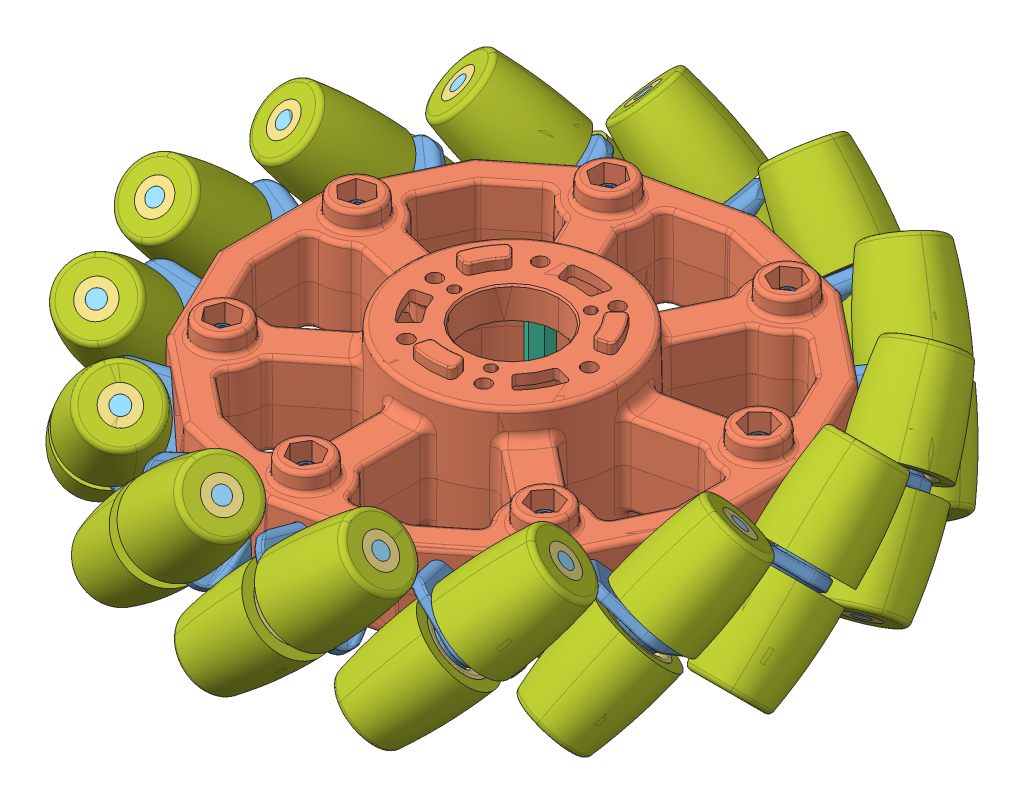
SolidWorks assembly 8_Mecanum_Wheel_Left_217-2801, configuration Default. Lengths in mm.
Overall size (213.38 67.99 218.38).
149 component instances, 10 part files, 0 mates.
Components (placement in the parent):
- 8_Mecanum_Wheel_Left_217-2801.STEP-1: 8_Mecanum_Wheel_Left_217-2801.STEP [Default] at origin size (213.38 67.99 218.38)
  - 217-2799-002 Rev1.STEP-1: 217-2799-002 Rev1.STEP [Default] at (67.5204 0 0) x (0 0 -1) z (1 0 0) size (26.84 25.28 30.1)
  - 217-2801-001 Rev1.STEP-1: 217-2801-001 Rev1.STEP [Default] at (-0.0396 6.3542 -0.0405) x (1 0 0) z (0 -1 0) size (148.4 152.01 28.7)
  - 217-2801-001 Rev1.STEP-2: 217-2801-001 Rev1.STEP [Default] at (-0.0396 -6.3458 -0.0405) x (-1 0 0) z (0 1 0) size (148.4 152.01 28.7)
  - 217-2586-003 Rev2.STEP-1: 217-2586-003 Rev2.STEP [Default] at (88.2976 -4.0062 4.0062) x (-0.854327 -0.367509 -0.367509) z (-0.519737 0.6041 0.6041) size (19.46 28.57 19.46)
  - 217-2586-003 Rev2.STEP-2: 217-2586-003 Rev2.STEP [Default] at (88.2976 4.0062 -4.0062) x (0.717269 -0.492709 -0.492709) z (0.696796 0.507186 0.507186) size (19.46 28.57 19.46)
  - 217-2586-005 Rev2.STEP-1: 217-2586-005 Rev2.STEP [Default] at (88.2976 -6.3286 6.3286) x (0 0.707107 -0.707107) z (0.473193 -0.622932 -0.622932) size (8.5 8 8)
  - 217-2586-005 Rev2.STEP-2: 217-2586-005 Rev2.STEP [Default] at (88.2976 6.3286 -6.3286) x (0 0.707107 -0.707107) z (0.707107 -0.5 -0.5) size (8.5 8 8)
  - 217-2586-007 Rev1.STEP-1: 217-2586-007 Rev1.STEP [Default] at (88.2976 0 0) x (0 0.707107 -0.707107) z (0.543569 -0.59352 -0.59352) size (61.72 5 5)
  - 217-2586-008 Rev1.STEP-1: 217-2586-008 Rev1.STEP [Default] at (-11.9459 2.5442 -20.6627) x (0.866025 0 -0.5) z (0 -1 0) size (7.33 6.35 31.75)
  - 217-2587-002 Rev2.STEP-1: 217-2587-002 Rev2.STEP [Default] at (88.2976 -0.3986 0.3986) x (-0.963241 0.189956 0.189956) z (-0.268638 -0.681114 -0.681114) size (26.1 28.56 26.1)
  - 217-2587-002 Rev2.STEP-2: 217-2587-002 Rev2.STEP [Default] at (88.2976 0.3986 -0.3986) x (0.779223 -0.443177 -0.443177) z (-0.626747 -0.550994 -0.550994) size (26.1 28.56 26.1)
  - NUT-832-NYLOCK.STEP-1: NUT-832-NYLOCK.STEP [Default] at (-49.6859 -13.6521 39.5511) x (-0.365341 0 0.930874) z (0.930874 0 0.365341) size (9.38 5.92 9.38)
  - PINL-M050-0012-S.STEP-1: PINL-M050-0012-S.STEP [Default] at (-69.318 -0.0958 -15.8528) x (0 -1 0) z (-0.272222 0 0.962235) size (12 5 5)
  - SCREW-832-1250.STEP-1: SCREW-832-1250.STEP [Default] at (-49.6859 14.914 39.5511) x (0 -1 0) z (-0.321403 0 -0.946943) size (37.06 8 10.03)
  - 217-2586-008 Rev1.STEP-2: 217-2586-008 Rev1.STEP [Default] at (-23.8521 2.5442 -0.0405) x (0 0 -1) z (0 -1 0) size (7.33 6.35 31.75)
  - 217-2586-008 Rev1.STEP-3: 217-2586-008 Rev1.STEP [Default] at (-11.9459 2.5442 20.5817) x (-0.866025 0 -0.5) z (0 -1 0) size (7.33 6.35 31.75)
  - 217-2586-008 Rev1.STEP-4: 217-2586-008 Rev1.STEP [Default] at (11.8666 2.5442 20.5817) x (-0.866025 0 0.5) z (0 -1 0) size (7.33 6.35 31.75)
  - 217-2586-008 Rev1.STEP-5: 217-2586-008 Rev1.STEP [Default] at (23.7729 2.5442 -0.0405) x (0 0 1) z (0 -1 0) size (7.33 6.35 31.75)
  - 217-2586-008 Rev1.STEP-6: 217-2586-008 Rev1.STEP [Default] at (11.8666 2.5442 -20.6627) x (0.866025 0 0.5) z (0 -1 0) size (7.33 6.35 31.75)
  - NUT-832-NYLOCK.STEP-2: NUT-832-NYLOCK.STEP [Default] at (-0.0396 -13.6521 63.4595) x (0.5 0 0.866025) z (0.866025 0 -0.5) size (9.38 5.92 9.38)
  - NUT-832-NYLOCK.STEP-3: NUT-832-NYLOCK.STEP [Default] at (49.6067 -13.6521 39.5511) x (0.988831 0 0.149042) z (0.149042 0 -0.988831) size (9.38 5.92 9.38)
  - NUT-832-NYLOCK.STEP-4: NUT-832-NYLOCK.STEP [Default] at (61.8683 -13.6521 -14.1706) x (0.733052 0 -0.680173) z (-0.680173 0 -0.733052) size (9.38 5.92 9.38)
  - NUT-832-NYLOCK.STEP-5: NUT-832-NYLOCK.STEP [Default] at (27.512 -13.6521 -57.252) x (-0.07473 0 -0.997204) z (-0.997204 0 0.07473) size (9.38 5.92 9.38)
  - NUT-832-NYLOCK.STEP-6: NUT-832-NYLOCK.STEP [Default] at (-27.5912 -13.6521 -57.252) x (-0.826239 0 -0.56332) z (-0.56332 0 0.826239) size (9.38 5.92 9.38)
  - NUT-832-NYLOCK.STEP-7: NUT-832-NYLOCK.STEP [Default] at (-61.9475 -13.6521 -14.1706) x (-0.955573 0 0.294755) z (0.294755 0 0.955573) size (9.38 5.92 9.38)
  - SCREW-832-1250.STEP-2: SCREW-832-1250.STEP [Default] at (-0.0396 14.914 63.4595) x (0 -1 0) z (-0.940741 0 -0.339126) size (37.06 8 10.03)
  - SCREW-832-1250.STEP-3: SCREW-832-1250.STEP [Default] at (49.6067 14.914 39.5511) x (0 -1 0) z (-0.851682 0 0.524059) size (37.06 8 10.03)
  - SCREW-832-1250.STEP-4: SCREW-832-1250.STEP [Default] at (61.8683 14.914 -14.1706) x (0 -1 0) z (-0.121289 0 0.992617) size (37.06 8 10.03)
  - SCREW-832-1250.STEP-5: SCREW-832-1250.STEP [Default] at (27.512 14.914 -57.252) x (0 -1 0) z (0.700437 0 0.713714) size (37.06 8 10.03)
  - SCREW-832-1250.STEP-6: SCREW-832-1250.STEP [Default] at (-27.5912 14.914 -57.252) x (0 -1 0) z (0.99472 0 -0.10263) size (37.06 8 10.03)
  - SCREW-832-1250.STEP-7: SCREW-832-1250.STEP [Default] at (-61.9475 14.914 -14.1706) x (0 -1 0) z (0.539958 0 -0.841692) size (37.06 8 10.03)
  - PINL-M050-0012-S.STEP-2: PINL-M050-0012-S.STEP [Default] at (-69.318 -0.0958 15.7719) x (0 -1 0) z (0.172235 0 0.985056) size (12 5 5)
  - PINL-M050-0012-S.STEP-3: PINL-M050-0012-S.STEP [Default] at (-55.5966 -0.0958 44.2647) x (0 -1 0) z (0.582578 0 0.812775) size (12 5 5)
  - PINL-M050-0012-S.STEP-4: PINL-M050-0012-S.STEP [Default] at (-30.8714 -0.0958 63.9824) x (0 -1 0) z (0.877534 0 0.479514) size (12 5 5)
  - PINL-M050-0012-S.STEP-5: PINL-M050-0012-S.STEP [Default] at (-0.0396 -0.0958 71.0195) x (0 -1 0) z (0.998684 0 0.051279) size (12 5 5)
  - PINL-M050-0012-S.STEP-6: PINL-M050-0012-S.STEP [Default] at (30.7922 -0.0958 63.9824) x (0 -1 0) z (0.922033 0 -0.387112) size (12 5 5)
  - PINL-M050-0012-S.STEP-7: PINL-M050-0012-S.STEP [Default] at (55.5173 -0.0958 44.2647) x (0 -1 0) z (0.662761 0 -0.748831) size (12 5 5)
  - PINL-M050-0012-S.STEP-8: PINL-M050-0012-S.STEP [Default] at (69.2388 -0.0958 15.7719) x (0 -1 0) z (0.272222 0 -0.962235) size (12 5 5)
  - PINL-M050-0012-S.STEP-9: PINL-M050-0012-S.STEP [Default] at (69.2388 -0.0958 -15.8528) x (0 -1 0) z (-0.172235 0 -0.985056) size (12 5 5)
  - PINL-M050-0012-S.STEP-10: PINL-M050-0012-S.STEP [Default] at (55.5173 -0.0958 -44.3457) x (0 -1 0) z (-0.582578 0 -0.812775) size (12 5 5)
  - PINL-M050-0012-S.STEP-11: PINL-M050-0012-S.STEP [Default] at (30.7922 -0.0958 -64.0633) x (0 -1 0) z (-0.877534 0 -0.479514) size (12 5 5)
  - PINL-M050-0012-S.STEP-12: PINL-M050-0012-S.STEP [Default] at (-0.0396 -0.0958 -71.1005) x (0 -1 0) z (-0.998684 0 -0.051279) size (12 5 5)
  - PINL-M050-0012-S.STEP-13: PINL-M050-0012-S.STEP [Default] at (-30.8714 -0.0958 -64.0633) x (0 -1 0) z (-0.922033 0 0.387112) size (12 5 5)
  - PINL-M050-0012-S.STEP-14: PINL-M050-0012-S.STEP [Default] at (-55.5966 -0.0958 -44.3457) x (0 -1 0) z (-0.662761 0 0.748831) size (12 5 5)
  - 217-2587-002 Rev2.STEP-3: 217-2587-002 Rev2.STEP [Default] at (79.3941 0.3986 -38.6912) x (0.509769 -0.443177 -0.737381) z (-0.803746 -0.550994 -0.224493) size (26.1 28.56 26.1)
  - 217-2587-002 Rev2.STEP-4: 217-2587-002 Rev2.STEP [Default] at (54.7578 0.3986 -69.3286) x (0.139348 -0.443177 -0.885537) z (-0.821555 -0.550994 0.146471) size (26.1 28.56 26.1)
  - 217-2587-002 Rev2.STEP-5: 217-2587-002 Rev2.STEP [Default] at (19.2682 0.3986 -86.2426) x (-0.258672 -0.443177 -0.858303) z (-0.676644 -0.550994 0.488425) size (26.1 28.56 26.1)
  - 217-2587-002 Rev2.STEP-6: 217-2587-002 Rev2.STEP [Default] at (-20.0456 0.3986 -86.0832) x (-0.605459 -0.443177 -0.66107) z (-0.397715 -0.550994 0.73364) size (26.1 28.56 26.1)
  - 217-2587-002 Rev2.STEP-7: 217-2587-002 Rev2.STEP [Default] at (-55.3969 0.3986 -68.882) x (-0.832327 -0.443177 -0.332905) z (-0.040014 -0.550994 0.833549) size (26.1 28.56 26.1)
  - 217-2587-002 Rev2.STEP-8: 217-2587-002 Rev2.STEP [Default] at (-79.784 0.3986 -38.0459) x (-0.894343 -0.443177 0.061196) z (0.325612 -0.550994 0.768364) size (26.1 28.56 26.1)
  - 217-2587-002 Rev2.STEP-9: 217-2587-002 Rev2.STEP [Default] at (-88.3768 0.3986 0.3176) x (-0.779223 -0.443177 0.443177) z (0.626747 -0.550994 0.550994) size (26.1 28.56 26.1)
  - 217-2587-002 Rev2.STEP-10: 217-2587-002 Rev2.STEP [Default] at (-79.4733 0.3986 38.6102) x (-0.509769 -0.443177 0.737381) z (0.803746 -0.550994 0.224493) size (26.1 28.56 26.1)
  - 217-2587-002 Rev2.STEP-11: 217-2587-002 Rev2.STEP [Default] at (-54.837 0.3986 69.2476) x (-0.139348 -0.443177 0.885537) z (0.821555 -0.550994 -0.146471) size (26.1 28.56 26.1)
  - 217-2587-002 Rev2.STEP-12: 217-2587-002 Rev2.STEP [Default] at (-19.3474 0.3986 86.1616) x (0.258672 -0.443177 0.858303) z (0.676644 -0.550994 -0.488425) size (26.1 28.56 26.1)
  - 217-2587-002 Rev2.STEP-13: 217-2587-002 Rev2.STEP [Default] at (19.9664 0.3986 86.0022) x (0.605459 -0.443177 0.66107) z (0.397715 -0.550994 -0.73364) size (26.1 28.56 26.1)
  - 217-2587-002 Rev2.STEP-14: 217-2587-002 Rev2.STEP [Default] at (55.3177 0.3986 68.8011) x (0.832327 -0.443177 0.332905) z (0.040014 -0.550994 -0.833549) size (26.1 28.56 26.1)
  - 217-2587-002 Rev2.STEP-15: 217-2587-002 Rev2.STEP [Default] at (79.7048 0.3986 37.965) x (0.894343 -0.443177 -0.061196) z (-0.325612 -0.550994 -0.768364) size (26.1 28.56 26.1)
  - 217-2587-002 Rev2.STEP-16: 217-2587-002 Rev2.STEP [Default] at (79.74 -0.3986 -37.973) x (-0.785432 0.189956 0.589079) z (-0.537559 -0.681114 -0.497105) size (26.1 28.56 26.1)
  - 217-2587-002 Rev2.STEP-17: 217-2587-002 Rev2.STEP [Default] at (55.381 -0.3986 -68.8315) x (-0.452058 0.189956 0.871528) z (-0.70001 -0.681114 -0.214638) size (26.1 28.56 26.1)
  - 217-2587-002 Rev2.STEP-18: 217-2587-002 Rev2.STEP [Default] at (20.0453 -0.3986 -86.0652) x (-0.029148 0.189956 0.98136) z (-0.723815 -0.681114 0.110341) size (26.1 28.56 26.1)
  - 217-2587-002 Rev2.STEP-19: 217-2587-002 Rev2.STEP [Default] at (-19.2684 -0.3986 -86.2606) x (0.399535 0.189956 0.896822) z (-0.60426 -0.681114 0.413465) size (26.1 28.56 26.1)
  - 217-2587-002 Rev2.STEP-20: 217-2587-002 Rev2.STEP [Default] at (-54.7737 -0.3986 -69.379) x (0.749084 0.189956 0.634657) z (-0.365024 -0.681114 0.634698) size (26.1 28.56 26.1)
  - 217-2587-002 Rev2.STEP-21: 217-2587-002 Rev2.STEP [Default] at (-79.4382 -0.3986 -38.7641) x (0.950269 0.189956 0.24679) z (-0.05349 -0.681114 0.730221) size (26.1 28.56 26.1)
  - 217-2587-002 Rev2.STEP-22: 217-2587-002 Rev2.STEP [Default] at (-88.3768 -0.3986 -0.4795) x (0.963241 0.189956 -0.189956) z (0.268638 -0.681114 0.681114) size (26.1 28.56 26.1)
  - 217-2587-002 Rev2.STEP-23: 217-2587-002 Rev2.STEP [Default] at (-79.8192 -0.3986 37.892) x (0.785432 0.189956 -0.589079) z (0.537559 -0.681114 0.497105) size (26.1 28.56 26.1)
  - 217-2587-002 Rev2.STEP-24: 217-2587-002 Rev2.STEP [Default] at (-55.4602 -0.3986 68.7506) x (0.452058 0.189956 -0.871528) z (0.70001 -0.681114 0.214638) size (26.1 28.56 26.1)
  - 217-2587-002 Rev2.STEP-25: 217-2587-002 Rev2.STEP [Default] at (-20.1245 -0.3986 85.9842) x (0.029148 0.189956 -0.98136) z (0.723815 -0.681114 -0.110341) size (26.1 28.56 26.1)
  - 217-2587-002 Rev2.STEP-26: 217-2587-002 Rev2.STEP [Default] at (19.1892 -0.3986 86.1796) x (-0.399535 0.189956 -0.896822) z (0.60426 -0.681114 -0.413465) size (26.1 28.56 26.1)
  - 217-2587-002 Rev2.STEP-27: 217-2587-002 Rev2.STEP [Default] at (54.6945 -0.3986 69.2981) x (-0.749084 0.189956 -0.634657) z (0.365024 -0.681114 -0.634698) size (26.1 28.56 26.1)
  - 217-2587-002 Rev2.STEP-28: 217-2587-002 Rev2.STEP [Default] at (79.359 -0.3986 38.6832) x (-0.950269 0.189956 -0.24679) z (0.05349 -0.681114 -0.730221) size (26.1 28.56 26.1)
  - 217-2586-007 Rev1.STEP-2: 217-2586-007 Rev1.STEP [Default] at (79.567 0 -38.3321) x (-0.306802 0.707107 -0.637081) z (0.23222 -0.59352 -0.770589) size (61.72 5 5)
  - 217-2586-007 Rev1.STEP-3: 217-2586-007 Rev1.STEP [Default] at (55.0694 0 -69.08) x (-0.552838 0.707107 -0.440874) z (-0.125123 -0.59352 -0.795033) size (61.72 5 5)
  - 217-2586-007 Rev1.STEP-4: 217-2586-007 Rev1.STEP [Default] at (19.6567 0 -86.1539) x (-0.689378 0.707107 -0.157346) z (-0.457684 -0.59352 -0.662011) size (61.72 5 5)
  - 217-2586-007 Rev1.STEP-5: 217-2586-007 Rev1.STEP [Default] at (-19.657 0 -86.1719) x (-0.689378 0.707107 0.157346) z (-0.699595 -0.59352 -0.39787) size (61.72 5 5)
  - 217-2586-007 Rev1.STEP-6: 217-2586-007 Rev1.STEP [Default] at (-55.0853 0 -69.1305) x (-0.552838 0.707107 0.440874) z (-0.802943 -0.59352 -0.054926) size (61.72 5 5)
  - 217-2586-007 Rev1.STEP-7: 217-2586-007 Rev1.STEP [Default] at (-79.6111 0 -38.405) x (-0.306802 0.707107 0.637081) z (-0.747258 -0.59352 0.298897) size (61.72 5 5)
  - 217-2586-007 Rev1.STEP-8: 217-2586-007 Rev1.STEP [Default] at (-88.3768 0 -0.081) x (0 0.707107 0.707107) z (-0.543569 -0.59352 0.59352) size (61.72 5 5)
  - 217-2586-007 Rev1.STEP-9: 217-2586-007 Rev1.STEP [Default] at (-79.6462 0 38.2511) x (0.306802 0.707107 0.637081) z (-0.23222 -0.59352 0.770589) size (61.72 5 5)
  - 217-2586-007 Rev1.STEP-10: 217-2586-007 Rev1.STEP [Default] at (-55.1486 0 68.9991) x (0.552838 0.707107 0.440874) z (0.125123 -0.59352 0.795033) size (61.72 5 5)
  - 217-2586-007 Rev1.STEP-11: 217-2586-007 Rev1.STEP [Default] at (-19.736 0 86.0729) x (0.689378 0.707107 0.157346) z (0.457684 -0.59352 0.662011) size (61.72 5 5)
  - 217-2586-007 Rev1.STEP-12: 217-2586-007 Rev1.STEP [Default] at (19.5778 0 86.0909) x (0.689378 0.707107 -0.157346) z (0.699595 -0.59352 0.39787) size (61.72 5 5)
  - 217-2586-007 Rev1.STEP-13: 217-2586-007 Rev1.STEP [Default] at (55.0061 0 69.0496) x (0.552838 0.707107 -0.440874) z (0.802943 -0.59352 0.054926) size (61.72 5 5)
  - 217-2586-007 Rev1.STEP-14: 217-2586-007 Rev1.STEP [Default] at (79.5319 0 38.3241) x (0.306802 0.707107 -0.637081) z (0.747258 -0.59352 -0.298897) size (61.72 5 5)
  - 217-2586-005 Rev2.STEP-3: 217-2586-005 Rev2.STEP [Default] at (76.8211 6.3286 -44.034) x (-0.306802 0.707107 -0.637081) z (0.420139 -0.5 -0.757287) size (8.5 8 8)
  - 217-2586-005 Rev2.STEP-4: 217-2586-005 Rev2.STEP [Default] at (50.1215 6.3286 -73.0259) x (-0.552838 0.707107 -0.440874) z (0.049958 -0.5 -0.864583) size (8.5 8 8)
  - 217-2586-005 Rev2.STEP-5: 217-2586-005 Rev2.STEP [Default] at (13.4868 6.3286 -87.5621) x (-0.689378 0.707107 -0.157346) z (-0.330118 -0.5 -0.800639) size (8.5 8 8)
  - 217-2586-005 Rev2.STEP-6: 217-2586-005 Rev2.STEP [Default] at (-25.827 6.3286 -84.7636) x (-0.689378 0.707107 0.157346) z (-0.64481 -0.5 -0.578118) size (8.5 8 8)
  - 217-2586-005 Rev2.STEP-7: 217-2586-005 Rev2.STEP [Default] at (-60.0332 6.3286 -65.1847) x (-0.552838 0.707107 0.440874) z (-0.83179 -0.5 -0.241093) size (8.5 8 8)
  - 217-2586-005 Rev2.STEP-8: 217-2586-005 Rev2.STEP [Default] at (-82.357 6.3286 -32.7032) x (-0.306802 0.707107 0.637081) z (-0.854023 -0.5 0.143682) size (8.5 8 8)
  - 217-2586-005 Rev2.STEP-9: 217-2586-005 Rev2.STEP [Default] at (-88.3768 6.3286 6.2476) x (0 0.707107 0.707107) z (-0.707107 -0.5 0.5) size (8.5 8 8)
  - 217-2586-005 Rev2.STEP-10: 217-2586-005 Rev2.STEP [Default] at (-76.9004 6.3286 43.953) x (0.306802 0.707107 0.637081) z (-0.420139 -0.5 0.757287) size (8.5 8 8)
  - 217-2586-005 Rev2.STEP-11: 217-2586-005 Rev2.STEP [Default] at (-50.2007 6.3286 72.9449) x (0.552838 0.707107 0.440874) z (-0.049958 -0.5 0.864583) size (8.5 8 8)
  - 217-2586-005 Rev2.STEP-12: 217-2586-005 Rev2.STEP [Default] at (-13.566 6.3286 87.4812) x (0.689378 0.707107 0.157346) z (0.330118 -0.5 0.800639) size (8.5 8 8)
  - 217-2586-005 Rev2.STEP-13: 217-2586-005 Rev2.STEP [Default] at (25.7477 6.3286 84.6827) x (0.689378 0.707107 -0.157346) z (0.64481 -0.5 0.578118) size (8.5 8 8)
  - 217-2586-005 Rev2.STEP-14: 217-2586-005 Rev2.STEP [Default] at (59.954 6.3286 65.1037) x (0.552838 0.707107 -0.440874) z (0.83179 -0.5 0.241093) size (8.5 8 8)
  - 217-2586-005 Rev2.STEP-15: 217-2586-005 Rev2.STEP [Default] at (82.2778 6.3286 32.6222) x (0.306802 0.707107 -0.637081) z (0.854023 -0.5 -0.143682) size (8.5 8 8)
  - 217-2586-005 Rev2.STEP-16: 217-2586-005 Rev2.STEP [Default] at (82.3129 -6.3286 -32.6302) x (-0.306802 0.707107 -0.637081) z (0.156052 -0.622932 -0.766553) size (8.5 8 8)
  - 217-2586-005 Rev2.STEP-17: 217-2586-005 Rev2.STEP [Default] at (60.0173 -6.3286 -65.1342) x (-0.552838 0.707107 -0.440874) z (-0.191997 -0.622932 -0.758349) size (8.5 8 8)
  - 217-2586-005 Rev2.STEP-18: 217-2586-005 Rev2.STEP [Default] at (25.8267 -6.3286 -84.7456) x (-0.689378 0.707107 -0.157346) z (-0.502019 -0.622932 -0.599944) size (8.5 8 8)
  - 217-2586-005 Rev2.STEP-19: 217-2586-005 Rev2.STEP [Default] at (-13.4871 -6.3286 -87.5801) x (-0.689378 0.707107 0.157346) z (-0.712609 -0.622932 -0.322713) size (8.5 8 8)
  - 217-2586-005 Rev2.STEP-20: 217-2586-005 Rev2.STEP [Default] at (-50.1374 -6.3286 -73.0764) x (-0.552838 0.707107 0.440874) z (-0.782059 -0.622932 0.018435) size (8.5 8 8)
  - 217-2586-005 Rev2.STEP-21: 217-2586-005 Rev2.STEP [Default] at (-76.8652 -6.3286 -44.1069) x (-0.306802 0.707107 0.637081) z (-0.696612 -0.622932 0.355932) size (8.5 8 8)
  - 217-2586-005 Rev2.STEP-22: 217-2586-005 Rev2.STEP [Default] at (-88.3768 -6.3286 -6.4096) x (0 0.707107 0.707107) z (-0.473193 -0.622932 0.622932) size (8.5 8 8)
  - 217-2586-005 Rev2.STEP-23: 217-2586-005 Rev2.STEP [Default] at (-82.3921 -6.3286 32.5492) x (0.306802 0.707107 0.637081) z (-0.156052 -0.622932 0.766553) size (8.5 8 8)
  - 217-2586-005 Rev2.STEP-24: 217-2586-005 Rev2.STEP [Default] at (-60.0965 -6.3286 65.0533) x (0.552838 0.707107 0.440874) z (0.191997 -0.622932 0.758349) size (8.5 8 8)
  - 217-2586-005 Rev2.STEP-25: 217-2586-005 Rev2.STEP [Default] at (-25.9059 -6.3286 84.6647) x (0.689378 0.707107 0.157346) z (0.502019 -0.622932 0.599944) size (8.5 8 8)
  - 217-2586-005 Rev2.STEP-26: 217-2586-005 Rev2.STEP [Default] at (13.4079 -6.3286 87.4992) x (0.689378 0.707107 -0.157346) z (0.712609 -0.622932 0.322713) size (8.5 8 8)
  - 217-2586-005 Rev2.STEP-27: 217-2586-005 Rev2.STEP [Default] at (50.0582 -6.3286 72.9954) x (0.552838 0.707107 -0.440874) z (0.782059 -0.622932 -0.018435) size (8.5 8 8)
  - 217-2586-005 Rev2.STEP-28: 217-2586-005 Rev2.STEP [Default] at (76.786 -6.3286 44.0259) x (0.306802 0.707107 -0.637081) z (0.696612 -0.622932 -0.355932) size (8.5 8 8)
  - 217-2586-003 Rev2.STEP-3: 217-2586-003 Rev2.STEP [Default] at (77.8288 4.0062 -41.9416) x (0.432459 -0.492709 -0.755127) z (0.847851 0.507186 0.15463) size (19.46 28.57 19.46)
  - 217-2586-003 Rev2.STEP-4: 217-2586-003 Rev2.STEP [Default] at (51.9372 4.0062 -71.5779) x (0.061995 -0.492709 -0.867983) z (0.830979 0.507186 -0.228552) size (19.46 28.57 19.46)
  - 217-2586-003 Rev2.STEP-5: 217-2586-003 Rev2.STEP [Default] at (15.7509 4.0062 -87.0453) x (-0.320749 -0.492709 -0.808924) z (0.649521 0.507186 -0.566466) size (19.46 28.57 19.46)
  - 217-2586-003 Rev2.STEP-6: 217-2586-003 Rev2.STEP [Default] at (-23.5628 4.0062 -85.2804) x (-0.639963 -0.492709 -0.589648) z (0.339418 0.507186 -0.792185) size (19.46 28.57 19.46)
  - 217-2586-003 Rev2.STEP-7: 217-2586-003 Rev2.STEP [Default] at (-58.2175 4.0062 -66.6327) x (-0.832426 -0.492709 -0.253585) z (-0.037911 0.507186 -0.861002) size (19.46 28.57 19.46)
  - 217-2586-003 Rev2.STEP-8: 217-2586-003 Rev2.STEP [Default] at (-81.3494 4.0062 -34.7955) x (-0.860016 -0.492709 0.132704) z (-0.407732 0.507186 -0.759287) size (19.46 28.57 19.46)
  - 217-2586-003 Rev2.STEP-9: 217-2586-003 Rev2.STEP [Default] at (-88.3768 4.0062 3.9253) x (-0.717269 -0.492709 0.492709) z (-0.696796 0.507186 -0.507186) size (19.46 28.57 19.46)
  - 217-2586-003 Rev2.STEP-10: 217-2586-003 Rev2.STEP [Default] at (-77.908 4.0062 41.8606) x (-0.432459 -0.492709 0.755127) z (-0.847851 0.507186 -0.15463) size (19.46 28.57 19.46)
  - 217-2586-003 Rev2.STEP-11: 217-2586-003 Rev2.STEP [Default] at (-52.0164 4.0062 71.4969) x (-0.061995 -0.492709 0.867983) z (-0.830979 0.507186 0.228552) size (19.46 28.57 19.46)
  - 217-2586-003 Rev2.STEP-12: 217-2586-003 Rev2.STEP [Default] at (-15.8302 4.0062 86.9644) x (0.320749 -0.492709 0.808924) z (-0.649521 0.507186 0.566466) size (19.46 28.57 19.46)
  - 217-2586-003 Rev2.STEP-13: 217-2586-003 Rev2.STEP [Default] at (23.4836 4.0062 85.1995) x (0.639963 -0.492709 0.589648) z (-0.339418 0.507186 0.792185) size (19.46 28.57 19.46)
  - 217-2586-003 Rev2.STEP-14: 217-2586-003 Rev2.STEP [Default] at (58.1383 4.0062 66.5517) x (0.832426 -0.492709 0.253585) z (0.037911 0.507186 0.861002) size (19.46 28.57 19.46)
  - 217-2586-003 Rev2.STEP-15: 217-2586-003 Rev2.STEP [Default] at (81.2701 4.0062 34.7146) x (0.860016 -0.492709 -0.132704) z (0.407732 0.507186 0.759287) size (19.46 28.57 19.46)
  - 217-2586-003 Rev2.STEP-16: 217-2586-003 Rev2.STEP [Default] at (81.3053 -4.0062 -34.7226) x (-0.929178 -0.367509 0.039564) z (-0.206157 0.6041 0.769781) size (19.46 28.57 19.46)
  - 217-2586-003 Rev2.STEP-17: 217-2586-003 Rev2.STEP [Default] at (58.2016 -4.0062 -66.5822) x (-0.819994 -0.367509 0.438801) z (0.148254 0.6041 0.782997) size (19.46 28.57 19.46)
  - 217-2586-003 Rev2.STEP-18: 217-2586-003 Rev2.STEP [Default] at (23.5625 -4.0062 -85.2624) x (-0.548401 -0.367509 0.751128) z (0.473302 0.6041 0.641131) size (19.46 28.57 19.46)
  - 217-2586-003 Rev2.STEP-19: 217-2586-003 Rev2.STEP [Default] at (-15.7512 -4.0062 -87.0634) x (-0.16819 -0.367509 0.914685) z (0.704606 0.6041 0.372281) size (19.46 28.57 19.46)
  - 217-2586-003 Rev2.STEP-20: 217-2586-003 Rev2.STEP [Default] at (-51.9531 -4.0062 -71.6284) x (0.245334 -0.367509 0.897078) z (0.796355 0.6041 0.029696) size (19.46 28.57 19.46)
  - 217-2586-003 Rev2.STEP-21: 217-2586-003 Rev2.STEP [Default] at (-77.8729 -4.0062 -42.0145) x (0.610265 -0.367509 0.701793) z (0.730376 0.6041 -0.31877) size (19.46 28.57 19.46)
  - 217-2586-003 Rev2.STEP-22: 217-2586-003 Rev2.STEP [Default] at (-88.3768 -4.0062 -4.0872) x (0.854327 -0.367509 0.367509) z (0.519737 0.6041 -0.6041) size (19.46 28.57 19.46)
  - 217-2586-003 Rev2.STEP-23: 217-2586-003 Rev2.STEP [Default] at (-81.3845 -4.0062 34.6416) x (0.929178 -0.367509 -0.039564) z (0.206157 0.6041 -0.769781) size (19.46 28.57 19.46)
  - 217-2586-003 Rev2.STEP-24: 217-2586-003 Rev2.STEP [Default] at (-58.2808 -4.0062 66.5012) x (0.819994 -0.367509 -0.438801) z (-0.148254 0.6041 -0.782997) size (19.46 28.57 19.46)
  - 217-2586-003 Rev2.STEP-25: 217-2586-003 Rev2.STEP [Default] at (-23.6417 -4.0062 85.1814) x (0.548401 -0.367509 -0.751128) z (-0.473302 0.6041 -0.641131) size (19.46 28.57 19.46)
  - 217-2586-003 Rev2.STEP-26: 217-2586-003 Rev2.STEP [Default] at (15.672 -4.0062 86.9824) x (0.16819 -0.367509 -0.914685) z (-0.704606 0.6041 -0.372281) size (19.46 28.57 19.46)
  - 217-2586-003 Rev2.STEP-27: 217-2586-003 Rev2.STEP [Default] at (51.8739 -4.0062 71.5474) x (-0.245334 -0.367509 -0.897078) z (-0.796355 0.6041 -0.029696) size (19.46 28.57 19.46)
  - 217-2586-003 Rev2.STEP-28: 217-2586-003 Rev2.STEP [Default] at (77.7937 -4.0062 41.9336) x (-0.610265 -0.367509 -0.701793) z (-0.730376 0.6041 0.31877) size (19.46 28.57 19.46)
  - 217-2799-002 Rev1.STEP-2: 217-2799-002 Rev1.STEP [Default] at (60.8474 0 -29.3172) x (-0.433884 0 -0.900969) z (0.900969 0 -0.433884) size (26.84 25.28 30.1)
  - 217-2799-002 Rev1.STEP-3: 217-2799-002 Rev1.STEP [Default] at (42.115 0 -52.8358) x (-0.781831 0 -0.62349) z (0.62349 0 -0.781831) size (26.84 25.28 30.1)
  - 217-2799-002 Rev1.STEP-4: 217-2799-002 Rev1.STEP [Default] at (15.0334 0 -65.8976) x (-0.974928 0 -0.222521) z (0.222521 0 -0.974928) size (26.84 25.28 30.1)
  - 217-2799-002 Rev1.STEP-5: 217-2799-002 Rev1.STEP [Default] at (-15.0337 0 -65.9156) x (-0.974928 0 0.222521) z (-0.222521 0 -0.974928) size (26.84 25.28 30.1)
  - 217-2799-002 Rev1.STEP-6: 217-2799-002 Rev1.STEP [Default] at (-42.1309 0 -52.8863) x (-0.781831 0 0.62349) z (-0.62349 0 -0.781831) size (26.84 25.28 30.1)
  - 217-2799-002 Rev1.STEP-7: 217-2799-002 Rev1.STEP [Default] at (-60.8915 0 -29.3901) x (-0.433884 0 0.900969) z (-0.900969 0 -0.433884) size (26.84 25.28 30.1)
  - 217-2799-002 Rev1.STEP-8: 217-2799-002 Rev1.STEP [Default] at (-67.5996 0 -0.081) x (0 0 1) z (-1 0 0) size (26.84 25.28 30.1)
  - 217-2799-002 Rev1.STEP-9: 217-2799-002 Rev1.STEP [Default] at (-60.9266 0 29.2362) x (0.433884 0 0.900969) z (-0.900969 0 0.433884) size (26.84 25.28 30.1)
  - 217-2799-002 Rev1.STEP-10: 217-2799-002 Rev1.STEP [Default] at (-42.1942 0 52.7548) x (0.781831 0 0.62349) z (-0.62349 0 0.781831) size (26.84 25.28 30.1)
  - 217-2799-002 Rev1.STEP-11: 217-2799-002 Rev1.STEP [Default] at (-15.1126 0 65.8166) x (0.974928 0 0.222521) z (-0.222521 0 0.974928) size (26.84 25.28 30.1)
  - 217-2799-002 Rev1.STEP-12: 217-2799-002 Rev1.STEP [Default] at (14.9544 0 65.8347) x (0.974928 0 -0.222521) z (0.222521 0 0.974928) size (26.84 25.28 30.1)
  - 217-2799-002 Rev1.STEP-13: 217-2799-002 Rev1.STEP [Default] at (42.0517 0 52.8053) x (0.781831 0 -0.62349) z (0.62349 0 0.781831) size (26.84 25.28 30.1)
  - 217-2799-002 Rev1.STEP-14: 217-2799-002 Rev1.STEP [Default] at (60.8123 0 29.3092) x (0.433884 0 -0.900969) z (0.900969 0 0.433884) size (26.84 25.28 30.1)
